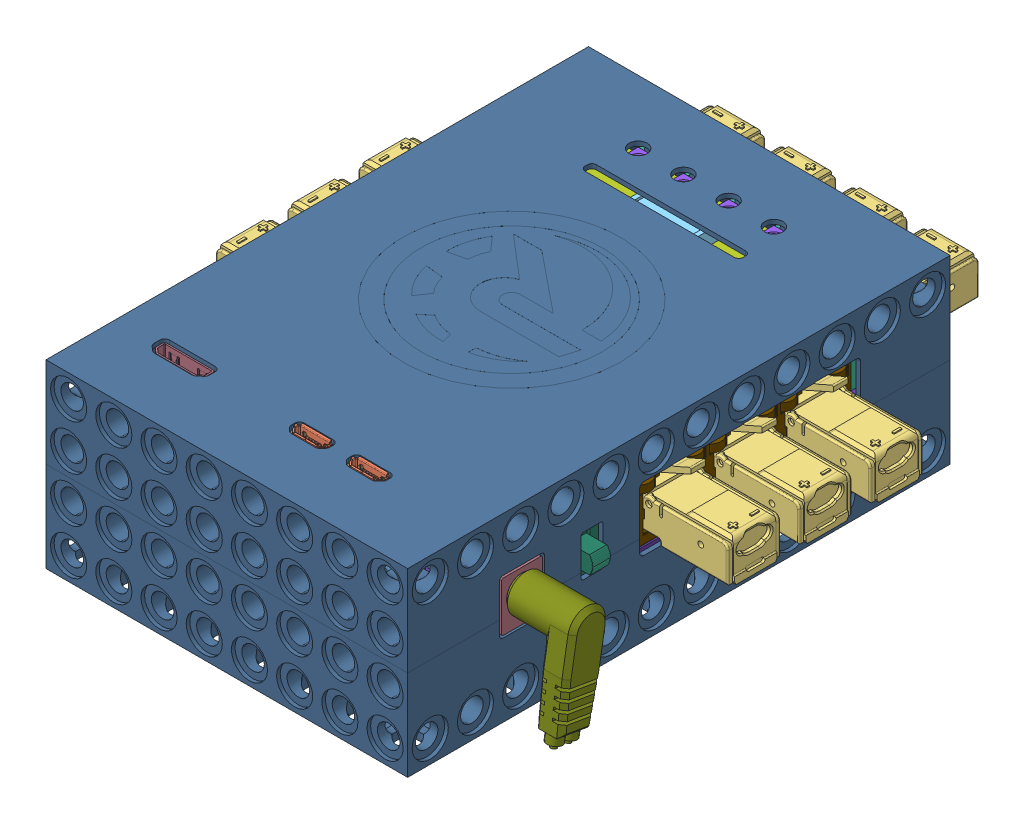
SolidWorks assembly PCBA_estimation_V2_JAN18, configuration Default. Lengths in mm.
Overall size (114.3 40.23 137.41).
125 component instances, 34 part files, 0 mates.
Components (placement in the parent):
- RapberryPiZero-1: RapberryPiZero [Default] at (82.9399 2.5974 70.7482) x (1 0 0) z (0 1 0) size (66.85 4.45 31.23)
  - Raspberry_pizero_PCB-1: Raspberry_pizero_PCB [Default] at (-51.2564 20.0966 13.0542) size (65 1 30)
  - Micro USB_input_female (short)-SMT-1: Micro USB_input_female (short)-SMT [Default] at (-42.3564 22.3216 26.5042) size (7.98 2.94 5.43)
  - Micro USB_input_female (short)-SMT-2: Micro USB_input_female (short)-SMT [Default] at (-29.7564 22.3216 26.5042) size (7.98 2.94 5.43)
  - 0204 - Capacitor-1: 0204 - Capacitor [Default] at (-62.4121 21.3466 11.2398) size (1.15 0.65 0.75)
  - 0204 - Capacitor-2: 0204 - Capacitor [Default] at (-62.4121 21.3466 12.2528) size (1.15 0.65 0.75)
  - 0204 - Capacitor-3: 0204 - Capacitor [Default] at (-61.8122 21.3466 13.3136) size (1.15 0.65 0.75)
  - 0204 - Capacitor-4: 0204 - Capacitor [Default] at (-61.8122 21.3466 14.2646) size (1.15 0.65 0.75)
  - 0204 - Capacitor-5: 0204 - Capacitor [Default] at (-61.8122 21.3466 15.241) size (1.15 0.65 0.75)
  - 0204 - Capacitor-6: 0204 - Capacitor [Default] at (-61.8122 21.3466 16.2144) size (1.15 0.65 0.75)
  - 0204 - Capacitor-7: 0204 - Capacitor [Default] at (-61.8122 21.3466 17.2416) size (1.15 0.65 0.75)
  - 0204 - Capacitor-8: 0204 - Capacitor [Default] at (-62.5919 21.3466 20.9695) size (1.15 0.65 0.75)
  - 0204 - Capacitor-9: 0204 - Capacitor [Default] at (-62.5919 21.3466 21.919) size (1.15 0.65 0.75)
  - 0204 - Capacitor-10: 0204 - Capacitor [Default] at (-60.4584 21.3466 22.3712) x (0 0 1) z (-1 0 0) size (1.15 0.65 0.75)
  - 0204 - Capacitor-11: 0204 - Capacitor [Default] at (-60.0807 21.3466 22.3712) x (0 0 -1) z (1 0 0) size (1.15 0.65 0.75)
  - 0204 - Capacitor-12: 0204 - Capacitor [Default] at (-59.0466 21.3466 22.3712) x (0 0 -1) z (1 0 0) size (1.15 0.65 0.75)
  - 0204 - Capacitor-13: 0204 - Capacitor [Default] at (-52.6496 21.3466 22.316) x (0 0 1) z (-1 0 0) size (1.15 0.65 0.75)
  - 0204 - Capacitor-14: 0204 - Capacitor [Default] at (-52.25 21.3466 22.316) x (0 0 -1) z (1 0 0) size (1.15 0.65 0.75)
  - 0204 - Capacitor-15: 0204 - Capacitor [Default] at (-51.2398 21.3466 22.316) x (0 0 -1) z (1 0 0) size (1.15 0.65 0.75)
  - 0204 - Capacitor-16: 0204 - Capacitor [Default] at (-49.1841 21.3466 22.316) x (0 0 -1) z (1 0 0) size (1.15 0.65 0.75)
  - 0204 - Capacitor-17: 0204 - Capacitor [Default] at (-48.1448 21.3466 22.316) x (0 0 -1) z (1 0 0) size (1.15 0.65 0.75)
  - 0204 - Capacitor-18: 0204 - Capacitor [Default] at (-46.475 21.3466 21.113) size (1.15 0.65 0.75)
  - 0204 - Capacitor-19: 0204 - Capacitor [Default] at (-45.7322 21.3466 20.0663) size (1.15 0.65 0.75)
  - 0204 - Capacitor-20: 0204 - Capacitor [Default] at (-45.7322 21.3466 19.0675) size (1.15 0.65 0.75)
  - 0204 - Capacitor-21: 0204 - Capacitor [Default] at (-45.7322 21.3466 18.1249) size (1.15 0.65 0.75)
  - 0204 - Capacitor-22: 0204 - Capacitor [Default] at (-45.7322 21.3466 17.1095) size (1.15 0.65 0.75)
  - 0204 - Capacitor-23: 0204 - Capacitor [Default] at (-46.3457 21.3466 16.1412) size (1.15 0.65 0.75)
  - 0204 - Capacitor-24: 0204 - Capacitor [Default] at (-46.3457 21.3466 15.1229) size (1.15 0.65 0.75)
  - 0204 - Capacitor-25: 0204 - Capacitor [Default] at (-46.3457 21.3466 14.0197) size (1.15 0.65 0.75)
  - 0204 - Capacitor-26: 0204 - Capacitor [Default] at (-46.3457 21.3466 12.9589) size (1.15 0.65 0.75)
  - 0204 - Capacitor-27: 0204 - Capacitor [Default] at (-43.6156 21.3466 13.1418) size (1.15 0.65 0.75)
  - 0204 - Capacitor-28: 0204 - Capacitor [Default] at (-43.6156 21.3466 10.1424) size (1.15 0.65 0.75)
  - 0204 - Capacitor-29: 0204 - Capacitor [Default] at (-48.9117 21.3466 7.6917) size (1.15 0.65 0.75)
  - 0204 - Capacitor-30: 0204 - Capacitor [Default] at (-55.4926 21.3466 7.2526) x (0 0 -1) z (1 0 0) size (1.15 0.65 0.75)
  - 0204 - Capacitor-31: 0204 - Capacitor [Default] at (-53.7932 21.3466 7.2526) x (0 0 1) z (-1 0 0) size (1.15 0.65 0.75)
  - 0204 - Capacitor-32: 0204 - Capacitor [Default] at (-59.8477 21.3466 7.2526) x (0 0 1) z (-1 0 0) size (1.15 0.65 0.75)
  - 0204- Resistor-1: 0204- Resistor [Default] at (-43.6109 21.4522 15.4193) x (-1 0 0) z (0 -1 0) size (0.99 0.51 0.36)
  - 0204- Resistor-2: 0204- Resistor [Default] at (-43.6109 21.4522 14.4127) x (-1 0 0) z (0 -1 0) size (0.99 0.51 0.36)
  - 0204- Resistor-3: 0204- Resistor [Default] at (-43.6109 21.4522 12.4047) x (-1 0 0) z (0 -1 0) size (0.99 0.51 0.36)
  - 0204- Resistor-4: 0204- Resistor [Default] at (-42.6936 21.4522 18.4076) x (-1 0 0) z (0 -1 0) size (0.99 0.51 0.36)
  - 0204- Resistor-5: 0204- Resistor [Default] at (-39.831 21.4522 18.1462) x (0 0 1) z (0 -1 0) size (0.99 0.51 0.36)
  - 0204- Resistor-6: 0204- Resistor [Default] at (-61.8169 21.4522 19.8533) x (-1 0 0) z (0 -1 0) size (0.99 0.51 0.36)
  - 0204- Resistor-7: 0204- Resistor [Default] at (-61.8169 21.4522 18.5178) x (-1 0 0) z (0 -1 0) size (0.99 0.51 0.36)
  - 0204- Resistor-8: 0204- Resistor [Default] at (-79.148 21.4522 17.7279) x (-1 0 0) z (0 -1 0) size (0.99 0.51 0.36)
  - 0204- Resistor-9: 0204- Resistor [Default] at (-56.0985 21.4522 7.2479) x (0 0 -1) z (0 -1 0) size (0.99 0.51 0.36)
  - 0204- Resistor-10: 0204- Resistor [Default] at (-28.0827 21.4522 9.5819) x (-1 0 0) z (0 -1 0) size (0.99 0.51 0.36)
  - CAP-0306-1: CAP-0306 [Default] at (-45.8903 21.4966 8.7634) size (1.6 0.8 0.9)
  - CAP-0306-2: CAP-0306 [Default] at (-82.0031 21.4966 19.0464) x (0 0 1) z (-1 0 0) size (1.6 0.8 0.9)
  - Raspberry_pizero_BCM2835 with VC4-1: Raspberry_pizero_BCM2835 with VC4 [Default] at (-54.1608 21.5466 15.1238) x (1 0 0) z (0 0 -1) size (12 0.65 12)
  - Crystal 3.4x2.4mm-1: Crystal 3.4x2.4mm [Default] at (-65.3089 21.0966 19.2633) size (3.2 1 2.4)
  - 0204- Resistor-11: 0204- Resistor [Default] at (-68.4329 21.4522 5.4384) x (0 0 1) z (0 -1 0) size (0.99 0.51 0.36)
  - 0204- Resistor-12: 0204- Resistor [Default] at (-69.7255 21.4522 5.4384) x (0 0 1) z (0 -1 0) size (0.99 0.51 0.36)
  - 0204- Resistor-13: 0204- Resistor [Default] at (-65.0626 21.4522 16.5355) x (1 0 0) z (0 -1 0) size (0.99 0.51 0.36)
  - 32,768 Khz Crystal-1: 32,768 Khz Crystal [Default] at (-60.5154 21.1428 26.5473) x (0.999848 -0.017452 0) z (0 0 1) size (3.4 1.03 1.5)
  - 0805- Capacitor-1: 0805- Capacitor [Default] at (-51.9496 21.9966 5.2384) x (1 0 0) z (0 -1 0) size (2 1.25 0.9)
  - 0805- Capacitor-2: 0805- Capacitor [Default] at (-51.9496 21.9966 7.3589) x (1 0 0) z (0 -1 0) size (2 1.25 0.9)
  - 0805- Capacitor-3: 0805- Capacitor [Default] at (-37.009 21.9966 22.5384) x (0 0 -1) z (0 -1 0) size (2 1.25 0.9)
  - 0805- Capacitor-4: 0805- Capacitor [Default] at (-29.8247 21.9966 13.3538) x (0 0 1) z (0 -1 0) size (2 1.25 0.9)
  - 0805- Capacitor-5: 0805- Capacitor [Default] at (-27.9052 21.9966 13.3538) x (0 0 -1) z (0 -1 0) size (2 1.25 0.9)
  - 0805- Capacitor-6: 0805- Capacitor [Default] at (-22.8003 21.9966 13.3538) x (0 0 -1) z (0 -1 0) size (2 1.25 0.9)
  - 0204- Resistor-14: 0204- Resistor [Default] at (-48.8769 21.4522 23.8207) x (1 0 0) z (0 -1 0) size (0.99 0.51 0.36)
  - 0204- Resistor-15: 0204- Resistor [Default] at (-52.4165 21.4522 24.0419) x (1 0 0) z (0 -1 0) size (0.99 0.51 0.36)
  - 0204 - Capacitor-33: 0204 - Capacitor [Default] at (-47.1199 21.3466 23.926) x (0 0 1) z (-1 0 0) size (1.15 0.65 0.75)
  - 0204 - Capacitor Brown-1: 0204 - Capacitor Brown [Default] at (-57.5817 21.3466 26.803) size (1.15 0.65 0.75)
  - 0204 - Capacitor Brown-2: 0204 - Capacitor Brown [Default] at (-64.0312 21.3466 26.8794) size (1.15 0.65 0.75)
  - 0204 - Capacitor Brown-3: 0204 - Capacitor Brown [Default] at (-46.3457 21.3466 12.214) size (1.15 0.65 0.75)
  - 0204 - Capacitor Brown-4: 0204 - Capacitor Brown [Default] at (-46.3457 21.3466 11.0963) size (1.15 0.65 0.75)
  - 0204 - Capacitor Brown-5: 0204 - Capacitor Brown [Default] at (-46.3457 21.3466 10.1566) size (1.15 0.65 0.75)
  - 0204 - Capacitor Brown-6: 0204 - Capacitor Brown [Default] at (-43.6156 21.3466 11.1151) size (1.15 0.65 0.75)
  - 0204 - Capacitor Brown-7: 0204 - Capacitor Brown [Default] at (-28.0874 21.3466 10.3236) size (1.15 0.65 0.75)
  - 0204 - Capacitor Brown-8: 0204 - Capacitor Brown [Default] at (-80.6197 21.3466 20.6997) size (1.15 0.65 0.75)
  - 0204- Resistor-16: 0204- Resistor [Default] at (-78.9105 21.4522 21.1554) x (1 0 0) z (0 -1 0) size (0.99 0.51 0.36)
  - 6-Pin SOT-1: 6-Pin SOT [Default] at (-79.714 21.0966 19.2138) x (0 0 1) z (0 1 0) size (1.5 1.84 0.95)
  - micro sd molex-1: micro sd molex [Default] at (-74.7768 21.6766 -33.0961) x (0 0 1) z (0 1 0) size (11.95 11.4 1.45)
  - hdmi type C-1: hdmi type C [Default] at (-71.3564 22.9466 28.6542) size (12.9 4.05 7.7)
  - Voltage Regulator 3x3mm 12-Pin-1: Voltage Regulator 3x3mm 12-Pin [Default] at (-23.6842 21.0966 12.6105) x (1 0 0) z (0 1 0) size (3 4.1 1.2)
  - 1210 inductor-1: 1210 inductor [Default] at (-46.4963 21.0916 6.3909) x (0 0 1) z (0 1 0) size (3.28 2.67 0.72)
  - 1210 inductor-2: 1210 inductor [Default] at (-28.2854 21.0916 17.6682) x (1 0 0) z (0 1 0) size (3.28 2.67 0.72)
  - 0204 - Capacitor-34: 0204 - Capacitor [Default] at (-48.9117 21.3466 6.5273) size (1.15 0.65 0.75)
  - 545482271-1: 545482271 [Default] at (-21.4564 21.1166 13.0542) x (0 0 -1) z (1 0 0) size (16.2 1.2 5)
- Motherboard_PCB-1: Motherboard_PCB [Default] at (6.6241 6.68 -16.7213) x (1 0 0) z (0 1 0) size (77 102.7 1.6)
- FCI_RJHSE538103-REVT1-1: FCI_RJHSE538103-REVT1 [Default] at (-1.6132 8.8896 3.0203) x (0 0 1) z (-1 0 0) size (51.17 18.92 16.61)
- TE_7-146256-0-1: TE_7-146256-0 [Default] at (31.6806 4.14 47.3655) x (1 0 0) z (0 0 -1) size (50.39 4.88 11.18)
- FCI_RJHSE538103-REVT1-2: FCI_RJHSE538103-REVT1 [Default] at (74.9804 8.8896 -28.2217) x (0 0 -1) z (1 0 0) size (51.17 18.92 16.61)
- QFP100P50_1600X1600X120L60X22-1: QFP100P50_1600X1600X120L60X22 [Default] at (34.1902 8.28 19.4603) x (1 0 0) z (0 1 0) size (16 16 1.21)
- 17x8669_2213145-2-1: 17x8669_2213145-2 [Default] at (64.9514 13.6886 3.2743) x (0 0 1) z (-1 0 0) size (11.7 14.58 29.91)
- Molex_1051330001-1: Molex_1051330001 [Default] at (1.5831 11.049 22.5312) x (0.008727 0 -0.999962) z (0 -1 0) size (8.01 3.02 9.01)
- PUI_AUDIO_AS01508AO-SC-WP-R-1: PUI_AUDIO_AS01508AO-SC-WP-R [Default] at (36.6836 27.6516 -33.8485) size (15 3 11)
- M-RJHSE-X38X-04-REVG1-1: M-RJHSE-X38X-04-REVG1 [Default] at (68.0526 8.661 -54.8913) x (-1 0 0) z (0 0 -1) size (66.95 18.85 17.2)
- LEDs_board_PCB-1: LEDs_board_PCB [Default] at (129.8284 155.5676 -9.1561) x (1 0 0) z (0 1 0) size (58 80 1.6)
- 11821-1: 11821 [Default] at (21.6836 27.8516 -42.8485) size (5.4 1.75 5)
- 11821-2: 11821 [Default] at (36.6836 27.8516 -21.8485) size (5.4 1.75 5)
- 11821-3: 11821 [Default] at (25.6836 27.8516 -18.901) x (0.866025 0 -0.5) z (0.5 0 0.866025) size (5.4 1.75 5)
- 11821-4: 11821 [Default] at (17.631 27.8516 -10.8485) x (0.5 0 -0.866025) z (0.866025 0 0.5) size (5.4 1.75 5)
- 11821-5: 11821 [Default] at (14.6836 27.8516 0.1515) x (0 0 -1) z (1 0 0) size (5.4 1.75 5)
- 11821-6: 11821 [Default] at (17.631 27.8516 11.1515) x (-0.5 0 -0.866025) z (0.866025 0 -0.5) size (5.4 1.75 5)
- 11821-7: 11821 [Default] at (25.6836 27.8516 19.2041) x (-0.866025 0 -0.5) z (0.5 0 -0.866025) size (5.4 1.75 5)
- 11821-8: 11821 [Default] at (36.6836 27.8516 22.1515) x (-1 0 0) z (0 0 -1) size (5.4 1.75 5)
- 11821-9: 11821 [Default] at (47.6836 27.8516 19.2041) x (-0.866025 0 0.5) z (-0.5 0 -0.866025) size (5.4 1.75 5)
- 11821-10: 11821 [Default] at (55.7361 27.8516 11.1515) x (-0.5 0 0.866025) z (-0.866025 0 -0.5) size (5.4 1.75 5)
- 11821-11: 11821 [Default] at (58.6836 27.8516 0.1515) x (0 0 1) z (-1 0 0) size (5.4 1.75 5)
- TSSOP-24[12-12]_0.45_0.65_5.6x7.8x1.6-1: TSSOP-24[12-12]_0.45_0.65_5.6x7.8x1.6 [Default] at (35.9825 8.28 -35.3299) x (1 0 0) z (0 1 0) size (7.8 7.6 1.6)
- TSSOP-24[12-12]_0.45_0.65_5.6x7.8x1.6-2: TSSOP-24[12-12]_0.45_0.65_5.6x7.8x1.6 [Default] at (47.6895 8.28 -14.9941) x (-0.008727 0 0.999962) z (0 1 0) size (7.8 7.6 1.6)
- TSSOP-24[12-12]_0.45_0.65_5.6x7.8x1.6-3: TSSOP-24[12-12]_0.45_0.65_5.6x7.8x1.6 [Default] at (20.9757 8.28 -17.9597) x (-0.008727 0 0.999962) z (0 1 0) size (7.8 7.6 1.6)
- BRcA-1: BRcA [Default] at (36.6836 -8.3484 3.1515) x (0 0 -1) z (1 0 0) size (120 40 80)
- Micro SD Card-1: Micro SD Card [Default] at (-3.3164 19.4408 48.3871) x (0 -1 0) z (-1 0 0) size (11.21 1.12 15.03)
- JHY_813270_2000mAh-1: JHY_813270_2000mAh [Default] at (37.0596 17.9516 23.8986) x (1 0 0) z (0 1 0) size (32 70.5 8.1)
- CUI_INC_PJ-037A-1: CUI_INC_PJ-037A [Default] at (76.6836 8.28 37.8515) x (0 0 -1) z (1 0 0) size (9 14.5 14.5)
- _ _ _C202LJBN-RC-1: _ _ _C202LJBN-RC [Default] at (57.3306 6.68 38.8655) x (-1 0 0) z (0 1 0) size (51.3 12.84 8.23)
- 11821-12: 11821 [Default] at (31.6836 27.8516 -42.8485) size (5.4 1.75 5)
- 11821-13: 11821 [Default] at (41.6836 27.8516 -42.8485) size (5.4 1.75 5)
- 11821-14: 11821 [Default] at (51.6836 27.8516 -42.8485) size (5.4 1.75 5)
- 11821-15: 11821 [Default] at (55.7361 27.8516 -10.8485) x (0.5 0 0.866025) z (-0.866025 0 0.5) size (5.4 1.75 5)
- 11821-16: 11821 [Default] at (47.6836 27.8516 -18.901) x (0.866025 0 0.5) z (-0.5 0 0.866025) size (5.4 1.75 5)
- 500SDPxS1M7xEA-1: 500SDPxS1M7xEA [Default] at (66.2036 14.63 22.3515) x (0 -1 0) z (1 0 0) size (15.88 11.43 25.96)
- Power_Jack_2mm-1: Power_Jack_2mm [Default] at (91.9336 14.78 37.8515) x (0 0.985977 -0.166882) z (0 0.166882 0.985977) size (26 26.35 8.3)
- 17x8669_2213145-2-2: 17x8669_2213145-2 [Default] at (64.9514 13.6886 -12.4737) x (0 0 1) z (-1 0 0) size (11.7 14.58 29.91)
- 17x8669_2213145-2-3: 17x8669_2213145-2 [Default] at (64.9514 13.6886 -28.2217) x (0 0 1) z (-1 0 0) size (11.7 14.58 29.91)
- 17x8669_2213145-2-4: 17x8669_2213145-2 [Default] at (8.4158 13.6886 3.0203) x (0 0 -1) z (1 0 0) size (11.7 14.58 29.91)
- 17x8669_2213145-2-5: 17x8669_2213145-2 [Default] at (8.4158 13.6886 -12.7277) x (0 0 -1) z (1 0 0) size (11.7 14.58 29.91)
- 17x8669_2213145-2-6: 17x8669_2213145-2 [Default] at (8.4158 13.6886 -28.4757) x (0 0 -1) z (1 0 0) size (11.7 14.58 29.91)
- 17x8669_2213145-2-7: 17x8669_2213145-2 [Default] at (60.1786 13.6886 -45.3782) size (11.7 14.58 29.91)
- 17x8669_2213145-2-8: 17x8669_2213145-2 [Default] at (44.4306 13.6886 -45.3782) size (11.7 14.58 29.91)
- 17x8669_2213145-2-9: 17x8669_2213145-2 [Default] at (28.6826 13.6886 -45.3782) size (11.7 14.58 29.91)
- 17x8669_2213145-2-10: 17x8669_2213145-2 [Default] at (12.9346 13.6886 -45.3782) size (11.7 14.58 29.91)
